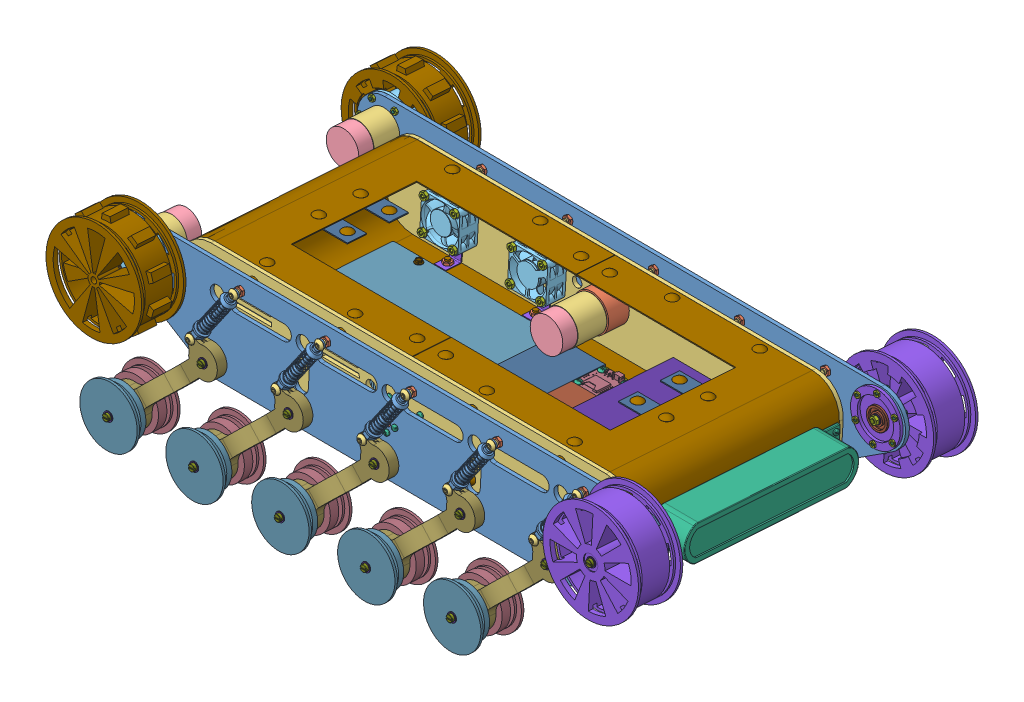
SolidWorks assembly Ensamble_Detallado_2, configuration Predeterminado. Lengths in mm. (continued)
Components (placement in the parent): (continued)
- hex nut jam_am-43: hex nut jam_am [B18.2.4.5M - Hex jam nut,  M5 x 0.8 --D-N] at (0.8451 27.9052 -764.5414) x (0.998432 -0.003331 -0.055871) z (0.000029 -0.998197 0.06003) size (8 9.24 2.7)
- Pieza_union_chasis-12: Pieza_union_chasis [Predeterminado] at (0.8279 31.0583 -773.7475) x (0.999983 0.000382 0.005859) z (-0.005872 0.060029 0.998179) size (12 20 17)
- hex nut jam_am-44: hex nut jam_am [B18.2.4.5M - Hex jam nut,  M5 x 0.8 --D-N] at (0.8224 19.1399 -772.029) x (0.997689 0.06792 0.001784) z (0.005872 -0.060029 -0.998179) size (8 9.24 2.7)
- round head bolt_ai-44: round head bolt_ai [RHBOLT 0.19-24x0.25x0.25-N] at (0.8673 18.6812 -779.6567) x (-0.005872 0.060029 0.998179) z (0 0.998197 -0.06003) size (8.99 11.53 11.53)
- hex nut style 1 gradeab_bsi-9: hex nut style 1 gradeab_bsi [BS EN 24032 - M4 - W - N] at (17.1747 7.9624 -749.0201) x (0.984097 -0.176868 0.016425) z (-0.005872 0.060029 0.998179) size (7 8.08 3.2)
- fillister head tapping screw_ai-9: fillister head tapping screw_ai [FHTS 0.151-19-slot-AB-1.125-N] at (17.3484 6.1863 -778.5539) x (-0.005872 0.060029 0.998179) z (-0.999983 -0.000176 -0.005872) size (31.66 6.3 6.3)
- fillister head tapping screw_ai-10: fillister head tapping screw_ai [FHTS 0.151-19-slot-AB-1.125-N] at (-14.651 6.1807 -778.7418) x (-0.005872 0.060029 0.998179) z (-0.999983 -0.000176 -0.005872) size (31.66 6.3 6.3)
- hex nut style 1 gradeab_bsi-10: hex nut style 1 gradeab_bsi [BS EN 24032 - M4 - W - N] at (-14.8248 7.9568 -749.208) x (0.58545 -0.809033 0.052098) z (-0.005872 0.060029 0.998179) size (7 8.08 3.2)
- fan-3: fan [По умолчанию] at (1.3081 -10.733 -771.2315) x (-0.999983 -0.000176 -0.005872) z (-0.005872 0.060029 0.998179) size (41.13 41.33 20.18)
- fan-4: fan [По умолчанию] at (-90.8077 -9.5136 -751.8102) x (0.999983 0.000176 0.005872) z (0.005872 -0.060029 -0.998179) size (41.13 41.33 20.18)
- round head bolt_ai-45: round head bolt_ai [RHBOLT 0.19-24x0.25x0.25-N] at (-91.2211 18.6461 -780.1963) x (-0.005872 0.060029 0.998179) z (0 0.998197 -0.06003) size (8.99 11.53 11.53)
- hex nut jam_am-45: hex nut jam_am [B18.2.4.5M - Hex jam nut,  M5 x 0.8 --D-N] at (-91.266 19.1048 -772.5686) x (0.997689 0.06792 0.001784) z (0.005872 -0.060029 -0.998179) size (8 9.24 2.7)
- Pieza_union_chasis-13: Pieza_union_chasis [Predeterminado] at (-91.2605 31.0231 -774.2871) x (0.999983 0.000382 0.005859) z (-0.005872 0.060029 0.998179) size (12 20 17)
- hex nut jam_am-46: hex nut jam_am [B18.2.4.5M - Hex jam nut,  M5 x 0.8 --D-N] at (-91.2433 27.8701 -765.081) x (0.998432 -0.003331 -0.055871) z (0.000029 -0.998197 0.06003) size (8 9.24 2.7)
- round head bolt_ai-46: round head bolt_ai [RHBOLT 0.19-24x0.25x0.25-N] at (-91.2435 35.0365 -765.512) x (0.000029 -0.998197 0.06003) z (-0.011742 0.060025 0.998128) size (8.99 11.53 11.53)
- round head bolt_ai-47: round head bolt_ai [RHBOLT 0.19-24x0.25x0.25-N] at (-82.6701 39.5021 -691.2612) x (0.000029 -0.998197 0.06003) z (-0.011742 0.060025 0.998128) size (8.99 11.53 11.53)
- hex nut jam_am-47: hex nut jam_am [B18.2.4.5M - Hex jam nut,  M5 x 0.8 --D-N] at (-82.6699 32.1737 -690.8205) x (0.965072 -0.015699 -0.261515) z (0.000029 -0.998197 0.06003) size (8 9.24 2.7)
- lamina_union-5: lamina_union [Predeterminado] at (-97.6697 34.8631 -691.0704) x (0.005872 -0.060029 -0.998179) z (-0.000029 0.998197 -0.06003) size (20 50 1)
- round head bolt_ai-48: round head bolt_ai [RHBOLT 0.19-24x0.25x0.25-N] at (-112.6696 39.4906 -691.437) x (0.000029 -0.998197 0.06003) z (-0.011742 0.060025 0.998128) size (8.99 11.53 11.53)
- hex nut jam_am-48: hex nut jam_am [B18.2.4.5M - Hex jam nut,  M5 x 0.8 --D-N] at (-112.6694 32.1623 -690.9962) x (0.919846 0.023576 0.39157) z (0.000029 -0.998197 0.06003) size (8 9.24 2.7)
- Pared_chasis-3: Pared_chasis [Predeterminado] at (69.8321 -14.1148 -774.6323) x (0.999983 -0.000205 0.005895) z (-0.005872 0.060029 0.998179) size (474 84 4)
- hex nut style 1 gradeab_bsi-11: hex nut style 1 gradeab_bsi [BS EN 24032 - M4 - W - N] at (-106.8044 7.7836 -752.9445) x (-0.99528 0.096345 -0.011649) z (0.005872 -0.060029 -0.998179) size (7 8.08 3.2)
- fillister head tapping screw_ai-11: fillister head tapping screw_ai [FHTS 0.151-19-slot-AB-1.125-N] at (-106.6494 6.1995 -779.2841) x (-0.005872 0.060029 0.998179) z (-0.999983 -0.000176 -0.005872) size (31.66 6.3 6.3)
- fillister head tapping screw_ai-12: fillister head tapping screw_ai [FHTS 0.151-19-slot-AB-1.125-N] at (-74.65 6.2052 -779.0962) x (-0.005872 0.060029 0.998179) z (-0.999983 -0.000176 -0.005872) size (31.66 6.3 6.3)
- hex nut style 1 gradeab_bsi-12: hex nut style 1 gradeab_bsi [BS EN 24032 - M4 - W - N] at (-74.8237 7.9813 -749.5624) x (0.58545 -0.809033 0.052098) z (-0.005872 0.060029 0.998179) size (7 8.08 3.2)
- hex nut style 1 gradeab_bsi-13: hex nut style 1 gradeab_bsi [BS EN 24032 - M4 - W - N] at (-106.8288 -23.9666 -747.8294) x (0.581467 0.8123 -0.04543) z (-0.005872 0.060029 0.998179) size (7 8.08 3.2)
- fillister head tapping screw_ai-13: fillister head tapping screw_ai [FHTS 0.151-19-slot-AB-1.125-N] at (-106.6551 -25.7428 -777.3631) x (-0.005872 0.060029 0.998179) z (-0.999983 -0.000176 -0.005872) size (31.66 6.3 6.3)
- hex nut style 1 gradeab_bsi-14: hex nut style 1 gradeab_bsi [BS EN 24032 - M4 - W - N] at (-74.8294 -23.961 -747.6415) x (0.984097 -0.176868 0.016425) z (-0.005872 0.060029 0.998179) size (7 8.08 3.2)
- fillister head tapping screw_ai-14: fillister head tapping screw_ai [FHTS 0.151-19-slot-AB-1.125-N] at (-74.6556 -25.7371 -777.1752) x (-0.005872 0.060029 0.998179) z (-0.999983 -0.000176 -0.005872) size (31.66 6.3 6.3)
- round head bolt_ai-49: round head bolt_ai [RHBOLT 0.19-24x0.25x0.25-N] at (-91.2194 -39.5732 -776.6951) x (-0.005872 0.060029 0.998179) z (-0.000059 0.998197 -0.06003) size (8.99 11.53 11.53)
- hex nut jam_am-49: hex nut jam_am [B18.2.4.5M - Hex jam nut,  M5 x 0.8 --D-N] at (-91.2801 -38.9524 -766.3723) x (0.997693 -0.067158 0.009908) z (-0.005872 0.060029 0.998179) size (8 9.24 2.7)
- Pieza_union_chasis-14: Pieza_union_chasis [Predeterminado] at (-91.2581 -51.1529 -769.3452) x (-0.999983 -0.000382 -0.005859) z (-0.005872 0.060029 0.998179) size (12 20 17)
- round head bolt_ai-50: round head bolt_ai [RHBOLT 0.19-24x0.25x0.25-N] at (-91.2409 -54.0857 -760.1523) x (-0.000029 0.998197 -0.06003) z (0.011742 -0.060025 -0.998128) size (8.99 11.53 11.53)
- hex nut jam_am-50: hex nut jam_am [B18.2.4.5M - Hex jam nut,  M5 x 0.8 --D-N] at (-91.241 -49.6144 -760.4212) x (0.998432 -0.003331 -0.055871) z (0.000029 -0.998197 0.06003) size (8 9.24 2.7)
- hex nut style 1 gradeab_bsi-15: hex nut style 1 gradeab_bsi [BS EN 24032 - M4 - W - N] at (-14.8304 -23.9855 -747.2871) x (-0.609484 -0.791576 0.044019) z (-0.005872 0.060029 0.998179) size (7 8.08 3.2)
- fillister head tapping screw_ai-15: fillister head tapping screw_ai [FHTS 0.151-19-slot-AB-1.125-N] at (-14.6567 -25.7616 -776.8208) x (-0.005872 0.060029 0.998179) z (-0.999983 -0.000176 -0.005872) size (31.66 6.3 6.3)
- fillister head tapping screw_ai-16: fillister head tapping screw_ai [FHTS 0.151-19-slot-AB-1.125-N] at (17.3428 -25.7559 -776.6329) x (-0.005872 0.060029 0.998179) z (-0.999983 -0.000176 -0.005872) size (31.66 6.3 6.3)
- hex nut style 1 gradeab_bsi-16: hex nut style 1 gradeab_bsi [BS EN 24032 - M4 - W - N] at (17.169 -23.9798 -747.0992) x (-0.609484 -0.791576 0.044019) z (-0.005872 0.060029 0.998179) size (7 8.08 3.2)
- round head bolt_ai-51: round head bolt_ai [RHBOLT 0.19-24x0.25x0.25-N] at (0.869 -39.538 -776.1555) x (-0.005872 0.060029 0.998179) z (-0.000059 0.998197 -0.06003) size (8.99 11.53 11.53)
- hex nut jam_am-51: hex nut jam_am [B18.2.4.5M - Hex jam nut,  M5 x 0.8 --D-N] at (0.8083 -38.9172 -765.8327) x (0.997693 -0.067158 0.009908) z (-0.005872 0.060029 0.998179) size (8 9.24 2.7)
- Pieza_union_chasis-15: Pieza_union_chasis [Predeterminado] at (0.8303 -51.1177 -768.8056) x (-0.999983 -0.000382 -0.005859) z (-0.005872 0.060029 0.998179) size (12 20 17)
- Motor_4-3: Motor_4 [Predeterminado] at (65.4869 10.5475 -728.8048) x (-0.994997 -0.099904 0.000155) z (0.005872 -0.060029 -0.998179) size (43.61 43.61 89.6)
  - Motor_1-1: Motor_1 [Predeterminado] at (-1.5658 -18.1483 21.75) size (36.8 36.8 43.5)
  - Motor_2-1: Motor_2 [Predeterminado] at (-1.5658 -18.1483 -8.95) x (-0.954241 0.299039 0) z (0 0 1) size (34.8 34.8 30.7)
  - Motor_3-1: Motor_3 [Predeterminado] at (-1.5658 -18.1483 -24.35) x (0.996313 -0.085794 0) z (0 0 1) size (34 34 15.4)
- round head bolt_ai-52: round head bolt_ai [RHBOLT 0.19-24x0.25x0.25-N] at (54.6994 35.7526 -753.6765) x (0.000029 -0.998197 0.06003) z (-0.011742 0.060025 0.998128) size (8.99 11.53 11.53)
- round head bolt_ai-53: round head bolt_ai [RHBOLT 0.19-24x0.25x0.25-N] at (84.6989 35.764 -753.5007) x (0.000029 -0.998197 0.06003) z (-0.011742 0.060025 0.998128) size (8.99 11.53 11.53)
- hex nut jam_am-52: hex nut jam_am [B18.2.4.5M - Hex jam nut,  M5 x 0.8 --D-N] at (84.6991 28.4357 -753.06) x (0.633352 0.046474 0.772467) z (0.000029 -0.998197 0.06003) size (8 9.24 2.7)
- hex nut jam_am-53: hex nut jam_am [B18.2.4.5M - Hex jam nut,  M5 x 0.8 --D-N] at (54.6996 28.4242 -753.2358) x (0.989604 -0.008604 -0.143563) z (0.000029 -0.998197 0.06003) size (8 9.24 2.7)
- lamina_union-6: lamina_union [Predeterminado] at (69.6993 32.1233 -753.37) x (-0.005872 0.060029 0.998179) z (0.000029 -0.998197 0.06003) size (20 50 1)
- hex nut jam_am-54: hex nut jam_am [B18.2.4.5M - Hex jam nut,  M5 x 0.8 --D-N] at (138.8427 27.877 -763.728) x (0.998432 -0.003331 -0.055871) z (0.000029 -0.998197 0.06003) size (8 9.24 2.7)
- Pieza_union_chasis-16: Pieza_union_chasis [Predeterminado] at (138.8255 31.03 -772.9341) x (0.999983 0.000382 0.005859) z (-0.005872 0.060029 0.998179) size (12 20 17)
- hex nut jam_am-55: hex nut jam_am [B18.2.4.5M - Hex jam nut,  M5 x 0.8 --D-N] at (138.82 19.1117 -771.2156) x (0.997689 0.06792 0.001784) z (0.005872 -0.060029 -0.998179) size (8 9.24 2.7)
- round head bolt_ai-54: round head bolt_ai [RHBOLT 0.19-24x0.25x0.25-N] at (138.8649 18.653 -778.8432) x (-0.005872 0.060029 0.998179) z (0 0.998197 -0.06003) size (8.99 11.53 11.53)
- round head bolt_ai-55: round head bolt_ai [RHBOLT 0.19-24x0.25x0.25-N] at (138.8425 35.0434 -764.1589) x (0.000029 -0.998197 0.06003) z (-0.011742 0.060025 0.998128) size (8.99 11.53 11.53)
- hex nut jam_am-56: hex nut jam_am [B18.2.4.5M - Hex jam nut,  M5 x 0.8 --D-N] at (251.3244 32.3013 -688.8634) x (0.998432 -0.003331 -0.055871) z (0.000029 -0.998197 0.06003) size (8 9.24 2.7)
- round head bolt_ai-56: round head bolt_ai [RHBOLT 0.19-24x0.25x0.25-N] at (251.3241 39.6296 -689.3042) x (0.000029 -0.998197 0.06003) z (-0.011742 0.060025 0.998128) size (8.99 11.53 11.53)
- hex nut jam_am-57: hex nut jam_am [B18.2.4.5M - Hex jam nut,  M5 x 0.8 --D-N] at (230.7712 27.8581 -763.1861) x (0.998432 -0.003331 -0.055871) z (0.000029 -0.998197 0.06003) size (8 9.24 2.7)
- hex nut jam_am-58: hex nut jam_am [B18.2.4.5M - Hex jam nut,  M5 x 0.8 --D-N] at (230.8184 19.0928 -770.6732) x (0.997689 0.06792 0.001784) z (0.005872 -0.060029 -0.998179) size (8 9.24 2.7)
- Pieza_union_chasis-17: Pieza_union_chasis [Predeterminado] at (230.8239 31.0112 -772.3918) x (0.999983 0.000382 0.005859) z (-0.005872 0.060029 0.998179) size (12 20 17)
- round head bolt_ai-57: round head bolt_ai [RHBOLT 0.19-24x0.25x0.25-N] at (230.771 35.1595 -763.6252) x (0.000029 -0.998197 0.06003) z (-0.011742 0.060025 0.998128) size (8.99 11.53 11.53)
- round head bolt_ai-58: round head bolt_ai [RHBOLT 0.19-24x0.25x0.25-N] at (221.3247 39.6182 -689.4799) x (0.000029 -0.998197 0.06003) z (-0.011742 0.060025 0.998128) size (8.99 11.53 11.53)
- round head bolt_ai-59: round head bolt_ai [RHBOLT 0.19-24x0.25x0.25-N] at (230.8633 18.6341 -778.3009) x (-0.005872 0.060029 0.998179) z (0 0.998197 -0.06003) size (8.99 11.53 11.53)
- hex nut jam_am-59: hex nut jam_am [B18.2.4.5M - Hex jam nut,  M5 x 0.8 --D-N] at (221.3249 32.2898 -689.0392) x (0.948595 -0.018971 -0.315922) z (0.000029 -0.998197 0.06003) size (8 9.24 2.7)
- lamina_union-7: lamina_union [Predeterminado] at (236.3245 34.9907 -689.1134) x (0.005872 -0.060029 -0.998179) z (-0.000029 0.998197 -0.06003) size (20 50 1)
- round head bolt_ai-60: round head bolt_ai [RHBOLT 0.19-24x0.25x0.25-N] at (230.865 -39.3152 -774.816) x (-0.005872 0.060029 0.998179) z (-0.000059 0.998197 -0.06003) size (8.99 11.53 11.53)
- hex nut jam_am-60: hex nut jam_am [B18.2.4.5M - Hex jam nut,  M5 x 0.8 --D-N] at (230.8043 -38.6945 -764.4932) x (0.997693 -0.067158 0.009908) z (-0.005872 0.060029 0.998179) size (8 9.24 2.7)
- Pieza_union_chasis-18: Pieza_union_chasis [Predeterminado] at (230.8263 -50.8949 -767.4661) x (-0.999983 -0.000382 -0.005859) z (-0.005872 0.060029 0.998179) size (12 20 17)
- round head bolt_ai-61: round head bolt_ai [RHBOLT 0.19-24x0.25x0.25-N] at (230.7736 -53.9627 -758.2655) x (-0.000029 0.998197 -0.06003) z (0.011742 -0.060025 -0.998128) size (8.99 11.53 11.53)
- hex nut jam_am-61: hex nut jam_am [B18.2.4.5M - Hex jam nut,  M5 x 0.8 --D-N] at (230.7735 -49.3565 -758.5425) x (0.998432 -0.003331 -0.055871) z (0.000029 -0.998197 0.06003) size (8 9.24 2.7)
- round head bolt_ai-62: round head bolt_ai [RHBOLT 0.19-24x0.25x0.25-N] at (138.8666 -39.4044 -775.3518) x (-0.005872 0.060029 0.998179) z (-0.000059 0.998197 -0.06003) size (8.99 11.53 11.53)
- hex nut jam_am-62: hex nut jam_am [B18.2.4.5M - Hex jam nut,  M5 x 0.8 --D-N] at (138.8059 -38.7836 -765.029) x (0.997693 -0.067158 0.009908) z (-0.005872 0.060029 0.998179) size (8 9.24 2.7)
- Pieza_union_chasis-19: Pieza_union_chasis [Predeterminado] at (138.8279 -50.984 -768.0019) x (-0.999983 -0.000382 -0.005859) z (-0.005872 0.060029 0.998179) size (12 20 17)
- round head bolt_ai-63: round head bolt_ai [RHBOLT 0.19-24x0.25x0.25-N] at (138.8452 -53.9169 -758.809) x (-0.000029 0.998197 -0.06003) z (0.011742 -0.060025 -0.998128) size (8.99 11.53 11.53)
- hex nut jam_am-63: hex nut jam_am [B18.2.4.5M - Hex jam nut,  M5 x 0.8 --D-N] at (138.845 -49.4456 -759.0779) x (0.998432 -0.003331 -0.055871) z (0.000029 -0.998197 0.06003) size (8 9.24 2.7)
- round head bolt_ai-64: round head bolt_ai [RHBOLT 0.19-24x0.25x0.25-N] at (0.8476 -54.0505 -759.6127) x (-0.000029 0.998197 -0.06003) z (0.011742 -0.060025 -0.998128) size (8.99 11.53 11.53)
- hex nut jam_am-64: hex nut jam_am [B18.2.4.5M - Hex jam nut,  M5 x 0.8 --D-N] at (0.8474 -49.5792 -759.8816) x (0.998432 -0.003331 -0.055871) z (0.000029 -0.998197 0.06003) size (8 9.24 2.7)
- pan head tapping screw_am-68: pan head tapping screw_am [PHT 3x10x9-slot-D-N] at (61.2159 3.7361 -777.9605) x (-0.005872 0.060029 0.998179) z (-0.00169 -0.998196 0.06002) size (12.2 5.6 5.6)
- pan head tapping screw_am-69: pan head tapping screw_am [PHT 3x10x9-slot-D-N] at (53.0101 -10.1356 -777.1746) x (-0.005872 0.060029 0.998179) z (0.865164 -0.500253 0.035174) size (12.2 5.6 5.6)
- pan head tapping screw_am-70: pan head tapping screw_am [PHT 3x10x9-slot-D-N] at (77.351 3.5825 -777.8564) x (-0.005872 0.060029 0.998179) z (-0.866854 -0.497942 0.024846) size (12.2 5.6 5.6)
- pan head tapping screw_am-71: pan head tapping screw_am [PHT 3x10x9-slot-D-N] at (85.2804 -10.4428 -776.9663) x (-0.005872 0.060029 0.998179) z (-0.865164 0.500253 -0.035174) size (12.2 5.6 5.6)
- pan head tapping screw_am-72: pan head tapping screw_am [PHT 3x10x9-slot-D-N] at (77.0746 -24.3145 -776.1803) x (-0.005872 0.060029 0.998179) z (0.00169 0.998196 -0.06002) size (12.2 5.6 5.6)
- pan head tapping screw_am-73: pan head tapping screw_am [PHT 3x10x9-slot-D-N] at (60.9395 -24.1609 -776.2845) x (-0.005872 0.060029 0.998179) z (0.866854 0.497942 -0.024846) size (12.2 5.6 5.6)
- Acople-2: Acople [Predeterminado] at (69.9159 -17.9828 -788.9757) x (-0.999983 0.000205 -0.005895) z (-0.005872 0.060029 0.998179) size (22 22 12)
- hex nut style 1_am-83: hex nut style 1_am [B18.2.4.1M - Hex nut, Style 1,  M3 x 0.5 --D-N] at (69.8945 -9.7331 -785.064) x (0.71889 -0.693604 0.045941) z (-0.005872 0.060029 0.998179) size (5.5 6.35 2.4)
- socket set screw cup point_ai-4: socket set screw cup point_ai [SSCUPSKT 0.125-44x0.125-HX-N] at (69.8776 -12.5716 -782.2886) x (-0.000558 -0.998197 0.060026) z (0.465529 0.052866 0.883452) size (3.17 3.17 3.17)
- hex nut style 1_am-84: hex nut style 1_am [B18.2.4.1M - Hex nut, Style 1,  M3 x 0.5 --D-N] at (61.8902 -17.7171 -784.6309) x (0.695099 0.717851 -0.039081) z (-0.005872 0.060029 0.998179) size (5.5 6.35 2.4)
- pan head tapping screw_am-74: pan head tapping screw_am [PHT 3x10x9-slot-D-N] at (61.9524 -18.3534 -795.2116) x (-0.005872 0.060029 0.998179) z (0.866854 0.497942 -0.024846) size (12.2 5.6 5.6)
- hex nut style 1_am-85: hex nut style 1_am [B18.2.4.1M - Hex nut, Style 1,  M3 x 0.5 --D-N] at (77.8899 -17.7203 -784.5366) x (-0.695099 -0.717851 0.039081) z (-0.005872 0.060029 0.998179) size (5.5 6.35 2.4)
- pan head tapping screw_am-75: pan head tapping screw_am [PHT 3x10x9-slot-D-N] at (77.9522 -18.3566 -795.1173) x (-0.005872 0.060029 0.998179) z (-0.866854 -0.497942 0.024846) size (12.2 5.6 5.6)
- pan head tapping screw_am-76: pan head tapping screw_am [PHT 3x10x9-slot-D-N] at (69.9568 -10.3694 -795.6447) x (-0.005872 0.060029 0.998179) z (0.498527 -0.86513 0.05496) size (12.2 5.6 5.6)
- pan head tapping screw_am-77: pan head tapping screw_am [PHT 3x10x9-slot-D-N] at (69.9478 -26.3406 -794.6842) x (-0.005872 0.060029 0.998179) z (0.498527 -0.86513 0.05496) size (12.2 5.6 5.6)
- hex nut style 1_am-86: hex nut style 1_am [B18.2.4.1M - Hex nut, Style 1,  M3 x 0.5 --D-N] at (69.8856 -25.7043 -784.1035) x (-0.71889 0.693604 -0.045941) z (-0.005872 0.060029 0.998179) size (5.5 6.35 2.4)
- Motor_4-4: Motor_4 [Predeterminado] at (-191.7252 26.7059 -775.4199) x (-0.999983 0.000205 -0.005895) z (0.005872 -0.060029 -0.998179) size (43.61 43.61 89.6)
  - Motor_1-1: Motor_1 [Predeterminado] at (-1.5658 -18.1483 21.75) size (36.8 36.8 43.5)
  - Motor_2-1: Motor_2 [Predeterminado] at (-1.5658 -18.1483 -8.95) x (-0.954241 0.299039 0) z (0 0 1) size (34.8 34.8 30.7)
  - Motor_3-1: Motor_3 [Predeterminado] at (-1.5658 -18.1483 -24.35) x (0.996313 -0.085794 0) z (0 0 1) size (34 34 15.4)
- hex nut style 1_am-87: hex nut style 1_am [B18.2.4.1M - Hex nut, Style 1,  M3 x 0.5 --D-N] at (-201.9536 28.1842 -790.947) x (0.275028 -0.959604 0.059327) z (-0.005872 0.060029 0.998179) size (5.5 6.35 2.4)
- hex nut style 1_am-88: hex nut style 1_am [B18.2.4.1M - Hex nut, Style 1,  M3 x 0.5 --D-N] at (-166.3398 7.6819 -789.5045) x (-0.970127 0.241753 -0.020245) z (-0.005872 0.060029 0.998179) size (5.5 6.35 2.4)
- pan head tapping screw_am-78: pan head tapping screw_am [PHT 3x10x9-slot-D-N] at (-166.2717 6.9856 -801.0834) x (-0.005872 0.060029 0.998179) z (-0.809274 -0.586638 0.030519) size (12.2 5.6 5.6)
- hex nut style 1_am-89: hex nut style 1_am [B18.2.4.1M - Hex nut, Style 1,  M3 x 0.5 --D-N] at (-178.214 28.1976 -790.8082) x (-0.695099 -0.717851 0.039081) z (-0.005872 0.060029 0.998179) size (5.5 6.35 2.4)
- pan head tapping screw_am-79: pan head tapping screw_am [PHT 3x10x9-slot-D-N] at (-178.1459 27.5013 -802.387) x (-0.005872 0.060029 0.998179) z (-0.104069 0.99274 -0.060314) size (12.2 5.6 5.6)
- pan head tapping screw_am-80: pan head tapping screw_am [PHT 3x10x9-slot-D-N] at (-201.8855 27.4878 -802.5259) x (-0.005872 0.060029 0.998179) z (0.913342 -0.406101 0.029795) size (12.2 5.6 5.6)
- hex nut style 1_am-90: hex nut style 1_am [B18.2.4.1M - Hex nut, Style 1,  M3 x 0.5 --D-N] at (-213.819 7.6551 -789.7822) x (0.970127 -0.241753 0.020245) z (-0.005872 0.060029 0.998179) size (5.5 6.35 2.4)
- pan head tapping screw_am-81: pan head tapping screw_am [PHT 3x10x9-slot-D-N] at (-213.7509 6.9587 -801.3611) x (-0.005872 0.060029 0.998179) z (0.809274 0.586638 -0.030519) size (12.2 5.6 5.6)
- hex nut style 1_am-91: hex nut style 1_am [B18.2.4.1M - Hex nut, Style 1,  M3 x 0.5 --D-N] at (-201.9448 -12.8606 -788.4786) x (0.695099 0.717851 -0.039081) z (-0.005872 0.060029 0.998179) size (5.5 6.35 2.4)
- pan head tapping screw_am-82: pan head tapping screw_am [PHT 3x10x9-slot-D-N] at (-201.8767 -13.5569 -800.0575) x (-0.005872 0.060029 0.998179) z (0.104069 -0.99274 0.060314) size (12.2 5.6 5.6)
- hex nut style 1_am-92: hex nut style 1_am [B18.2.4.1M - Hex nut, Style 1,  M3 x 0.5 --D-N] at (-178.2052 -12.8471 -788.3398) x (-0.275028 0.959604 -0.059327) z (-0.005872 0.060029 0.998179) size (5.5 6.35 2.4)
- pan head tapping screw_am-83: pan head tapping screw_am [PHT 3x10x9-slot-D-N] at (-201.8855 27.4878 -802.5259) x (-0.005872 0.060029 0.998179) z (-0.913342 0.406101 -0.029795) size (12.2 5.6 5.6)
- Rueda_TraseraV1.2-2: Rueda_TraseraV1.2 [Predeterminado] at (-190.0135 -0.0332 -801.1015) x (0.379256 -0.923487 0.057768) z (0.005872 -0.060029 -0.998179) size (100 100 46)
- Tapa_motor-2: Tapa_motor [Predeterminado] at (-189.898 5.8136 -820.4871) x (0.999983 -0.000205 0.005895) z (-0.005872 0.060029 0.998179) size (54.48 54.48 24.5)
- Pieza_Fijacion-2: Pieza_Fijacion [Predeterminado] at (329.5705 8.1054 -788.0154) x (0.999454 -0.032109 0.00781) z (0.005872 -0.060029 -0.998179) size (52 52 4)
- hex nut style 1_am-93: hex nut style 1_am [B18.2.4.1M - Hex nut, Style 1,  M3 x 0.5 --D-N] at (330.2763 30.8174 -784.9691) x (-0.437994 -0.897507 0.051398) z (-0.005872 0.060029 0.998179) size (5.5 6.35 2.4)
- hex nut style 1_am-94: hex nut style 1_am [B18.2.4.1M - Hex nut, Style 1,  M3 x 0.5 --D-N] at (309.7039 -2.2287 -783.1028) x (0.997518 0.070391 0.001635) z (-0.005872 0.060029 0.998179) size (5.5 6.35 2.4)
- hex nut style 1_am-95: hex nut style 1_am [B18.2.4.1M - Hex nut, Style 1,  M3 x 0.5 --D-N] at (310.4356 20.2191 -784.4484) x (0.559524 -0.827116 0.053033) z (-0.005872 0.060029 0.998179) size (5.5 6.35 2.4)
- pan head tapping screw_am-84: pan head tapping screw_am [PHT 3x10x9-slot-D-N] at (310.5095 19.4628 -797.0255) x (-0.005872 0.060029 0.998179) z (0.878463 0.477231 -0.023532) size (12.2 5.6 5.6)
- pan head tapping screw_am-85: pan head tapping screw_am [PHT 3x10x9-slot-D-N] at (309.7779 -2.985 -795.6798) x (-0.005872 0.060029 0.998179) z (0.025466 0.997882 -0.059861) size (12.2 5.6 5.6)
- pan head tapping screw_am-86: pan head tapping screw_am [PHT 3x10x9-slot-D-N] at (330.3503 30.061 -797.5462) x (-0.005872 0.060029 0.998179) z (0.852997 -0.520651 0.036329) size (12.2 5.6 5.6)
- pan head tapping screw_am-87: pan head tapping screw_am [PHT 3x10x9-slot-D-N] at (328.8869 -14.8346 -794.8548) x (-0.005872 0.060029 0.998179) z (-0.852997 0.520651 -0.036329) size (12.2 5.6 5.6)
- hex nut style 1_am-96: hex nut style 1_am [B18.2.4.1M - Hex nut, Style 1,  M3 x 0.5 --D-N] at (328.813 -14.0782 -782.2778) x (0.437994 0.897507 -0.051398) z (-0.005872 0.060029 0.998179) size (5.5 6.35 2.4)
- hex nut style 1_am-97: hex nut style 1_am [B18.2.4.1M - Hex nut, Style 1,  M4 x 0.7 --D-N] at (329.9033 7.646 -785.1807) x (-0.997796 0.065621 -0.009816) z (0.005872 -0.060029 -0.998179) size (7 8.08 3.2)
- plain washer - normal_as-7: plain washer - normal_as [AS 1237.1 N - 4] at (329.908 7.598 -785.9793) x (-0.998179 -0.060274 -0.002247) z (0.005872 -0.060029 -0.998179) size (9 9 0.8)
- cheese head screw_as-5: cheese head screw_as [AS-NZS 1427 CH - M4 x 60-N] at (330.248 4.1224 -843.7739) x (-0.005872 0.060029 0.998179) z (0.999978 0.003297 0.005684) size (62.62 7 7)
- instrument ball bearing_68_am-10: instrument ball bearing_68_am [AFBMA 12.1.4.1 - 0080-22 - 8,SI,NC,8_68] at (329.9285 7.3879 -789.4729) x (-0.005872 0.060029 0.998179) z (-0.436634 0.897859 -0.056564) size (7 22 22)
- hex nut style 1_am-98: hex nut style 1_am [B18.2.4.1M - Hex nut, Style 1,  M3 x 0.5 --D-N] at (349.3854 18.9678 -784.1441) x (-0.997518 -0.070391 -0.001635) z (-0.005872 0.060029 0.998179) size (5.5 6.35 2.4)
- hex nut style 1_am-99: hex nut style 1_am [B18.2.4.1M - Hex nut, Style 1,  M3 x 0.5 --D-N] at (348.6537 -3.48 -782.7984) x (-0.559524 0.827116 -0.053033) z (-0.005872 0.060029 0.998179) size (5.5 6.35 2.4)
- pan head tapping screw_am-88: pan head tapping screw_am [PHT 3x10x9-slot-D-N] at (349.4594 18.2115 -796.7211) x (-0.005872 0.060029 0.998179) z (-0.025466 -0.997882 0.059861) size (12.2 5.6 5.6)
- pan head tapping screw_am-89: pan head tapping screw_am [PHT 3x10x9-slot-D-N] at (348.7277 -4.2364 -795.3755) x (-0.005872 0.060029 0.998179) z (-0.878463 -0.477231 0.023532) size (12.2 5.6 5.6)
- Rueda_FrenteV1.2-3: Rueda_FrenteV1.2 [Predeterminado] at (329.9814 6.8477 -798.4565) x (-0.985592 0.168386 -0.015924) z (0.005872 -0.060029 -0.998179) size (100 100 48.5)
- Perfil_IzquierdoV2.2-2: Perfil_IzquierdoV2.2 [Predeterminado] at (69.9239 -24.6985 -790.5755) x (0.999983 -0.000205 0.005895) z (-0.005872 0.060029 0.998179) size (574.48 100.85 4)
- Tapa_Rueda_Delantera-2: Tapa_Rueda_Delantera [Predeterminado] at (329.955 7.1178 -793.9647) x (0.874162 0.485039 -0.024027) z (-0.005872 0.060029 0.998179) size (52 52 1)
- plain washer - normal_as-8: plain washer - normal_as [AS 1237.1 N - 4] at (330.2327 4.2784 -841.1786) x (-0.998179 -0.060274 -0.002247) z (0.005872 -0.060029 -0.998179) size (9 9 0.8)
- plain washer - normal_as-9: plain washer - normal_as [AS 1237.1 N - 4] at (330.2327 4.2784 -841.1786) x (-0.998179 -0.060274 -0.002247) z (0.005872 -0.060029 -0.998179) size (9 9 0.8)
- socket set screw cup point_ai-5: socket set screw cup point_ai [SSCUPSKT 0.125-44x0.125-HX-N] at (-195.3479 -4.5277 -837.9301) x (0.925273 0.378905 -0.017344) z (-0.170054 0.45527 0.873963) size (3.17 3.17 3.17)
- socket button head cap screw_am-4: socket button head cap screw_am [B18.3.4M - 5 x 0.8 x 16 SBHCS --N] at (272.2343 37.2025 -529.2777) x (0.005872 -0.060029 -0.998179) z (0.095597 -0.993591 0.060315) size (18.75 9.5 9.5)
- hex nut jam_am-65: hex nut jam_am [B18.2.4.5M - Hex jam nut,  M5 x 0.8 --D-N] at (273.7924 21.2739 -794.1446) x (0.998179 0.060274 0.002247) z (-0.005872 0.060029 0.998179) size (8 9.24 2.7)
- hex nut jam_am-66: hex nut jam_am [B18.2.4.5M - Hex jam nut,  M5 x 0.8 --D-N] at (273.753 21.6761 -787.4568) x (0.998179 0.060274 0.002247) z (-0.005872 0.060029 0.998179) size (8 9.24 2.7)
- hex nut jam_am-67: hex nut jam_am [B18.2.4.5M - Hex jam nut,  M5 x 0.8 --D-N] at (272.2787 36.7493 -536.8139) x (0.998179 0.060274 0.002247) z (-0.005872 0.060029 0.998179) size (8 9.24 2.7)
- hex nut jam_am-68: hex nut jam_am [B18.2.4.5M - Hex jam nut,  M5 x 0.8 --D-N] at (272.318 36.3471 -543.5017) x (0.998179 0.060274 0.002247) z (-0.005872 0.060029 0.998179) size (8 9.24 2.7)
- socket button head cap screw_am-7: socket button head cap screw_am [B18.3.4M - 5 x 0.8 x 16 SBHCS --N] at (273.8526 20.6586 -804.3759) x (-0.005872 0.060029 0.998179) z (0.095597 0.993658 -0.059195) size (18.75 9.5 9.5)
- instrument ball bearing_68_am-11: instrument ball bearing_68_am [AFBMA 12.1.4.1 - 0080-22 - 8,SI,NC,8_68] at (248.4008 -33.1814 -531.9474) x (-0.005872 0.060029 0.998179) z (0.539029 0.840952 -0.047403) size (7 22 22)
- Tubo_Pata-1: Tubo_Pata [Predeterminado] at (248.4448 -33.6316 -539.4338) x (0.999983 0.000176 0.005872) z (-0.005872 0.060029 0.998179) size (8 8 11)
- cheese head screw_as-6: cheese head screw_as [AS-NZS 1427 CH - M4 x 20-N] at (248.3339 -32.497 -520.5682) x (0.005872 -0.060029 -0.998179) z (-0.999978 -0.003297 -0.005684) size (22.6 7 7)
- plain washer - normal_as-10: plain washer - normal_as [AS 1237.1 N - 4] at (248.3538 -32.7011 -523.962) x (-0.998179 -0.060274 -0.002247) z (0.005872 -0.060029 -0.998179) size (9 9 0.8)
- hex nut style 1_am-101: hex nut style 1_am [B18.2.4.1M - Hex nut, Style 1,  M4 x 0.7 --D-N] at (248.4683 -33.8717 -543.4265) x (-0.99853 -0.054135 -0.002618) z (0.005872 -0.060029 -0.998179) size (7 8.08 3.2)
- plain washer - normal_as-11: plain washer - normal_as [AS 1237.1 N - 4] at (248.4495 -33.6796 -540.2323) x (0.958426 -0.284435 0.022743) z (0.005872 -0.060029 -0.998179) size (9 9 0.8)
- cheese head screw_as-7: cheese head screw_as [AS-NZS 1427 CH - M4 x 20-N] at (250.0067 -49.5992 -804.9495) x (-0.005872 0.060029 0.998179) z (0.11687 0.991397 -0.058933) size (22.6 7 7)
- hex nut style 1_am-102: hex nut style 1_am [B18.2.4.1M - Hex nut, Style 1,  M4 x 0.7 --D-N] at (249.891 -48.4167 -785.2854) x (-0.99853 -0.054135 -0.002618) z (0.005872 -0.060029 -0.998179) size (7 8.08 3.2)
- plain washer - normal_as-12: plain washer - normal_as [AS 1237.1 N - 4] at (249.8957 -48.4647 -786.0839) x (-0.998179 -0.060274 -0.002247) z (0.005872 -0.060029 -0.998179) size (9 9 0.8)
- plain washer - normal_as-13: plain washer - normal_as [AS 1237.1 N - 4] at (249.9914 -49.4432 -802.3542) x (0.958426 -0.284435 0.022743) z (0.005872 -0.060029 -0.998179) size (9 9 0.8)
- Rueda_Resorte2V1.3-15: Rueda_Resorte2V1.3 [Predeterminado] at (190.6052 -110.6664 -808.2385) x (0.047484 -0.997054 0.06024) z (-0.005872 0.060029 0.998179) size (60 60 20.5)
- Rueda_ResorteV1.3-19: Rueda_ResorteV1.3 [Predeterminado] at (190.6639 -111.2667 -818.2203) x (0.99997 -0.004709 0.006165) z (0.005872 -0.060029 -0.998179) size (60 60 17)
- plain washer - normal_as-14: plain washer - normal_as [AS 1237.1 N - 4] at (98.9726 -93.942 -530.9757) x (-0.998179 -0.060274 -0.002247) z (0.005872 -0.060029 -0.998179) size (9 9 0.8)
- plain washer - normal_as-15: plain washer - normal_as [AS 1237.1 N - 4] at (8.9742 -93.9235 -531.5062) x (-0.998179 -0.060274 -0.002247) z (0.005872 -0.060029 -0.998179) size (9 9 0.8)
- plain washer - normal_as-16: plain washer - normal_as [AS 1237.1 N - 4] at (-81.0242 -93.9051 -532.0367) x (-0.998179 -0.060274 -0.002247) z (0.005872 -0.060029 -0.998179) size (9 9 0.8)
- plain washer - normal_as-17: plain washer - normal_as [AS 1237.1 N - 4] at (-171.0227 -93.8867 -532.5672) x (-0.998179 -0.060274 -0.002247) z (0.005872 -0.060029 -0.998179) size (9 9 0.8)
- hex nut style 1_am-103: hex nut style 1_am [B18.2.4.1M - Hex nut, Style 1,  M4 x 0.7 --D-N] at (98.9914 -94.1341 -534.1698) x (-0.998179 -0.060274 -0.002247) z (0.005872 -0.060029 -0.998179) size (7 8.08 3.2)
- hex nut style 1_am-104: hex nut style 1_am [B18.2.4.1M - Hex nut, Style 1,  M4 x 0.7 --D-N] at (8.993 -94.1156 -534.7004) x (-0.998179 -0.060274 -0.002247) z (0.005872 -0.060029 -0.998179) size (7 8.08 3.2)
- hex nut style 1_am-105: hex nut style 1_am [B18.2.4.1M - Hex nut, Style 1,  M4 x 0.7 --D-N] at (-81.0054 -94.0972 -535.2309) x (-0.998179 -0.060274 -0.002247) z (0.005872 -0.060029 -0.998179) size (7 8.08 3.2)
- hex nut style 1_am-106: hex nut style 1_am [B18.2.4.1M - Hex nut, Style 1,  M4 x 0.7 --D-N] at (-171.0039 -94.0788 -535.7614) x (-0.998179 -0.060274 -0.002247) z (0.005872 -0.060029 -0.998179) size (7 8.08 3.2)
- plain washer - normal_as-18: plain washer - normal_as [AS 1237.1 N - 4] at (98.7066 -91.2227 -485.7581) x (-0.998179 -0.060274 -0.002247) z (0.005872 -0.060029 -0.998179) size (9 9 0.8)
- plain washer - normal_as-19: plain washer - normal_as [AS 1237.1 N - 4] at (8.7082 -91.2042 -486.2887) x (-0.998179 -0.060274 -0.002247) z (0.005872 -0.060029 -0.998179) size (9 9 0.8)
- plain washer - normal_as-20: plain washer - normal_as [AS 1237.1 N - 4] at (-81.2902 -91.1858 -486.8192) x (-0.998179 -0.060274 -0.002247) z (0.005872 -0.060029 -0.998179) size (9 9 0.8)
- plain washer - normal_as-21: plain washer - normal_as [AS 1237.1 N - 4] at (-171.2887 -91.1674 -487.3497) x (-0.998179 -0.060274 -0.002247) z (0.005872 -0.060029 -0.998179) size (9 9 0.8)
- cheese head screw_as-8: cheese head screw_as [AS-NZS 1427 CH - M4 x 50-N] at (98.6867 -91.0186 -482.3643) x (0.005872 -0.060029 -0.998179) z (-0.998179 -0.060274 -0.002247) size (52.62 7 7)
- cheese head screw_as-9: cheese head screw_as [AS-NZS 1427 CH - M4 x 50-N] at (8.6882 -91.0001 -482.8948) x (0.005872 -0.060029 -0.998179) z (-0.998179 -0.060274 -0.002247) size (52.62 7 7)
- cheese head screw_as-10: cheese head screw_as [AS-NZS 1427 CH - M4 x 50-N] at (-81.3102 -90.9817 -483.4254) x (0.005872 -0.060029 -0.998179) z (-0.998179 -0.060274 -0.002247) size (52.62 7 7)
- cheese head screw_as-11: cheese head screw_as [AS-NZS 1427 CH - M4 x 50-N] at (-171.3086 -90.9633 -483.9559) x (0.005872 -0.060029 -0.998179) z (-0.998179 -0.060274 -0.002247) size (52.62 7 7)
- Rueda_Resorte2V1.3-16: Rueda_Resorte2V1.3 [Predeterminado] at (98.8564 -92.7534 -511.2117) x (-0.998179 -0.060274 -0.002247) z (0.005872 -0.060029 -0.998179) size (60 60 20.5)
- Rueda_Resorte2V1.3-17: Rueda_Resorte2V1.3 [Predeterminado] at (8.8579 -92.735 -511.7422) x (-0.998179 -0.060274 -0.002247) z (0.005872 -0.060029 -0.998179) size (60 60 20.5)
- Rueda_Resorte2V1.3-18: Rueda_Resorte2V1.3 [Predeterminado] at (-81.1405 -92.7165 -512.2727) x (-0.998179 -0.060274 -0.002247) z (0.005872 -0.060029 -0.998179) size (60 60 20.5)
- Rueda_Resorte2V1.3-19: Rueda_Resorte2V1.3 [Predeterminado] at (-171.1389 -92.6981 -512.8033) x (-0.998179 -0.060274 -0.002247) z (0.005872 -0.060029 -0.998179) size (60 60 20.5)
- Rueda_ResorteV1.3-20: Rueda_ResorteV1.3 [Predeterminado] at (98.7977 -92.1531 -501.2299) x (-0.99968 0.024219 -0.007337) z (-0.005872 0.060029 0.998179) size (60 60 17)
- Rueda_ResorteV1.3-21: Rueda_ResorteV1.3 [Predeterminado] at (8.7992 -92.1347 -501.7604) x (-0.99968 0.024219 -0.007337) z (-0.005872 0.060029 0.998179) size (60 60 17)
- Rueda_ResorteV1.3-22: Rueda_ResorteV1.3 [Predeterminado] at (-81.1992 -92.1162 -502.291) x (-0.99968 0.024219 -0.007337) z (-0.005872 0.060029 0.998179) size (60 60 17)
- Rueda_ResorteV1.3-23: Rueda_ResorteV1.3 [Predeterminado] at (-171.1976 -92.0978 -502.8215) x (-0.99968 0.024219 -0.007337) z (-0.005872 0.060029 0.998179) size (60 60 17)
- plain washer - normal_as-22: plain washer - normal_as [AS 1237.1 N - 4] at (158.4511 -33.6612 -540.7628) x (0.958426 -0.284435 0.022743) z (0.005872 -0.060029 -0.998179) size (9 9 0.8)
- plain washer - normal_as-23: plain washer - normal_as [AS 1237.1 N - 4] at (68.4527 -33.6427 -541.2933) x (0.958426 -0.284435 0.022743) z (0.005872 -0.060029 -0.998179) size (9 9 0.8)
- plain washer - normal_as-24: plain washer - normal_as [AS 1237.1 N - 4] at (-21.5458 -33.6243 -541.8239) x (0.958426 -0.284435 0.022743) z (0.005872 -0.060029 -0.998179) size (9 9 0.8)
- plain washer - normal_as-25: plain washer - normal_as [AS 1237.1 N - 4] at (-111.5442 -33.6059 -542.3544) x (0.958426 -0.284435 0.022743) z (0.005872 -0.060029 -0.998179) size (9 9 0.8)
- hex nut style 1_am-107: hex nut style 1_am [B18.2.4.1M - Hex nut, Style 1,  M4 x 0.7 --D-N] at (158.4699 -33.8533 -543.957) x (-0.99853 -0.054135 -0.002618) z (0.005872 -0.060029 -0.998179) size (7 8.08 3.2)
- hex nut style 1_am-108: hex nut style 1_am [B18.2.4.1M - Hex nut, Style 1,  M4 x 0.7 --D-N] at (68.4715 -33.8348 -544.4875) x (-0.99853 -0.054135 -0.002618) z (0.005872 -0.060029 -0.998179) size (7 8.08 3.2)
- hex nut style 1_am-109: hex nut style 1_am [B18.2.4.1M - Hex nut, Style 1,  M4 x 0.7 --D-N] at (-21.527 -33.8164 -545.018) x (-0.99853 -0.054135 -0.002618) z (0.005872 -0.060029 -0.998179) size (7 8.08 3.2)
- hex nut style 1_am-110: hex nut style 1_am [B18.2.4.1M - Hex nut, Style 1,  M4 x 0.7 --D-N] at (-111.5254 -33.798 -545.5485) x (-0.99853 -0.054135 -0.002618) z (0.005872 -0.060029 -0.998179) size (7 8.08 3.2)
- instrument ball bearing_68_am-12: instrument ball bearing_68_am [AFBMA 12.1.4.1 - 0080-22 - 8,SI,NC,8_68] at (158.4024 -33.1629 -532.4779) x (-0.005872 0.060029 0.998179) z (0.539029 0.840952 -0.047403) size (7 22 22)
- instrument ball bearing_68_am-13: instrument ball bearing_68_am [AFBMA 12.1.4.1 - 0080-22 - 8,SI,NC,8_68] at (68.4039 -33.1445 -533.0085) x (-0.005872 0.060029 0.998179) z (0.539029 0.840952 -0.047403) size (7 22 22)
- instrument ball bearing_68_am-14: instrument ball bearing_68_am [AFBMA 12.1.4.1 - 0080-22 - 8,SI,NC,8_68] at (-21.5945 -33.1261 -533.539) x (-0.005872 0.060029 0.998179) z (0.539029 0.840952 -0.047403) size (7 22 22)
- instrument ball bearing_68_am-15: instrument ball bearing_68_am [AFBMA 12.1.4.1 - 0080-22 - 8,SI,NC,8_68] at (-111.5929 -33.1076 -534.0695) x (-0.005872 0.060029 0.998179) z (0.539029 0.840952 -0.047403) size (7 22 22)
- plain washer - normal_as-26: plain washer - normal_as [AS 1237.1 N - 4] at (158.3554 -32.6827 -524.4925) x (-0.998179 -0.060274 -0.002247) z (0.005872 -0.060029 -0.998179) size (9 9 0.8)
- plain washer - normal_as-27: plain washer - normal_as [AS 1237.1 N - 4] at (68.357 -32.6643 -525.023) x (-0.998179 -0.060274 -0.002247) z (0.005872 -0.060029 -0.998179) size (9 9 0.8)
- plain washer - normal_as-28: plain washer - normal_as [AS 1237.1 N - 4] at (-21.6415 -32.6458 -525.5535) x (-0.998179 -0.060274 -0.002247) z (0.005872 -0.060029 -0.998179) size (9 9 0.8)
- plain washer - normal_as-29: plain washer - normal_as [AS 1237.1 N - 4] at (-111.6399 -32.6274 -526.0841) x (-0.998179 -0.060274 -0.002247) z (0.005872 -0.060029 -0.998179) size (9 9 0.8)
- cheese head screw_as-12: cheese head screw_as [AS-NZS 1427 CH - M4 x 20-N] at (158.3354 -32.4786 -521.0987) x (0.005872 -0.060029 -0.998179) z (-0.999978 -0.003297 -0.005684) size (22.6 7 7)
- cheese head screw_as-13: cheese head screw_as [AS-NZS 1427 CH - M4 x 20-N] at (68.337 -32.4602 -521.6292) x (0.005872 -0.060029 -0.998179) z (-0.999978 -0.003297 -0.005684) size (22.6 7 7)
- cheese head screw_as-14: cheese head screw_as [AS-NZS 1427 CH - M4 x 20-N] at (-21.6614 -32.4417 -522.1597) x (0.005872 -0.060029 -0.998179) z (-0.999978 -0.003297 -0.005684) size (22.6 7 7)
- cheese head screw_as-15: cheese head screw_as [AS-NZS 1427 CH - M4 x 20-N] at (-111.6599 -32.4233 -522.6902) x (0.005872 -0.060029 -0.998179) z (-0.999978 -0.003297 -0.005684) size (22.6 7 7)
- Pieza_ResorteV1.5-7: Pieza_ResorteV1.5 [Predeterminado] at (98.827 -92.4532 -506.2208) x (-0.005872 0.060029 0.998179) z (-0.699298 -0.713776 0.038812) size (30 44.97 120)
- Pieza_ResorteV1.5-8: Pieza_ResorteV1.5 [Predeterminado] at (8.8286 -92.4348 -506.7513) x (-0.005872 0.060029 0.998179) z (-0.699298 -0.713776 0.038812) size (30 44.97 120)
- Pieza_ResorteV1.5-9: Pieza_ResorteV1.5 [Predeterminado] at (-81.1699 -92.4164 -507.2819) x (-0.005872 0.060029 0.998179) z (-0.699298 -0.713776 0.038812) size (30 44.97 120)
- Pieza_ResorteV1.5-10: Pieza_ResorteV1.5 [Predeterminado] at (-171.1683 -92.3979 -507.8124) x (-0.005872 0.060029 0.998179) z (-0.699298 -0.713776 0.038812) size (30 44.97 120)
- socket button head cap screw_am-8: socket button head cap screw_am [B18.3.4M - 5 x 0.8 x 10 SBHCS --N] at (144.1106 -18.5319 -522.6723) x (0.005872 -0.060029 -0.998179) z (-0.163306 0.984738 -0.060181) size (12.75 9.5 9.5)
- socket button head cap screw_am-9: socket button head cap screw_am [B18.3.4M - 5 x 0.8 x 10 SBHCS --N] at (54.1122 -18.5135 -523.2028) x (0.005872 -0.060029 -0.998179) z (-0.163306 0.984738 -0.060181) size (12.75 9.5 9.5)
- socket button head cap screw_am-10: socket button head cap screw_am [B18.3.4M - 5 x 0.8 x 10 SBHCS --N] at (-35.8863 -18.495 -523.7333) x (0.005872 -0.060029 -0.998179) z (-0.163306 0.984738 -0.060181) size (12.75 9.5 9.5)
- socket button head cap screw_am-11: socket button head cap screw_am [B18.3.4M - 5 x 0.8 x 10 SBHCS --N] at (-125.8847 -18.4766 -524.2638) x (0.005872 -0.060029 -0.998179) z (-0.163306 0.984738 -0.060181) size (12.75 9.5 9.5)
- Resorte-3: Resorte [Predeterminado] at (151.4618 -8.261 -531.0109) x (-0.827134 0.560678 -0.038584) z (-0.561974 -0.825855 0.04636) size (14 14 75.95)
- Resorte-4: Resorte [Predeterminado] at (61.4633 -8.2426 -531.5414) x (-0.827134 0.560678 -0.038584) z (-0.561974 -0.825855 0.04636) size (14 14 75.95)
- Resorte-5: Resorte [Predeterminado] at (-28.5351 -8.2242 -532.0719) x (-0.827134 0.560678 -0.038584) z (-0.561974 -0.825855 0.04636) size (14 14 75.95)
- Resorte-6: Resorte [Predeterminado] at (-118.5335 -8.2057 -532.6024) x (-0.827134 0.560678 -0.038584) z (-0.561974 -0.825855 0.04636) size (14 14 75.95)
- socket button head cap screw_am-12: socket button head cap screw_am [B18.3.4M - 5 x 0.8 x 16 SBHCS --N] at (182.2359 37.2209 -529.8082) x (0.005872 -0.060029 -0.998179) z (0.095597 -0.993591 0.060315) size (18.75 9.5 9.5)
- socket button head cap screw_am-13: socket button head cap screw_am [B18.3.4M - 5 x 0.8 x 16 SBHCS --N] at (92.2375 37.2394 -530.3387) x (0.005872 -0.060029 -0.998179) z (0.095597 -0.993591 0.060315) size (18.75 9.5 9.5)
- socket button head cap screw_am-14: socket button head cap screw_am [B18.3.4M - 5 x 0.8 x 16 SBHCS --N] at (2.239 37.2578 -530.8692) x (0.005872 -0.060029 -0.998179) z (0.095597 -0.993591 0.060315) size (18.75 9.5 9.5)
- socket button head cap screw_am-15: socket button head cap screw_am [B18.3.4M - 5 x 0.8 x 16 SBHCS --N] at (-87.7594 37.2762 -531.3997) x (0.005872 -0.060029 -0.998179) z (0.095597 -0.993591 0.060315) size (18.75 9.5 9.5)
